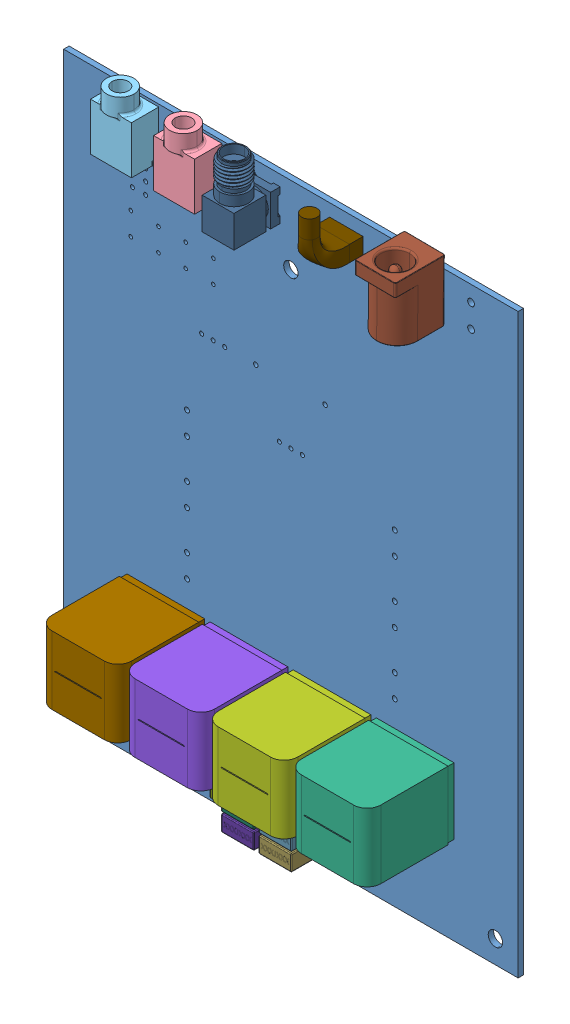
SolidWorks assembly CYAN_AMP_2, configuration 默认. Lengths in mm.
Overall size (100 132.86 23.29).
45 component instances, 18 part files, 2 mates.
Components (placement in the parent):
- CYAN_AMP_2(2)^CYAN_AMP_2-1: CYAN_AMP_2(2)^CYAN_AMP_2 [默认] at origin size (100 132.86 23.29) (virtual)
  - Board^CYAN_AMP_2(2)_CYAN_AMP_2-1: Board^CYAN_AMP_2(2)_CYAN_AMP_2 [默认] at (0 0 -0.8675) size (100 127 1.2) (virtual)
    - board-1: board [默认] at (0 0 -0.4115) size (100 127 1.2)
  - C34^CYAN_AMP_2(2)_CYAN_AMP_2-1: C34^CYAN_AMP_2(2)_CYAN_AMP_2 [默认] at origin (virtual)
    - C_0805^C34_CYAN_AMP_2(2)_CYAN_AMP_2-1: C_0805^C34_CYAN_AMP_2(2)_CYAN_AMP_2 [默认] at (8.9662 61.8782 -0.4115) x (0 1 0) z (0 0 -1) (virtual)
  - LED1^CYAN_AMP_2(2)_CYAN_AMP_2-1: LED1^CYAN_AMP_2(2)_CYAN_AMP_2 [默认] at origin size (3.2 1.6 1.01) (virtual)
    - LED_1206-R^LED1_CYAN_AMP_2(2)_CYAN_AMP_2-1: LED_1206-R^LED1_CYAN_AMP_2(2)_CYAN_AMP_2 [默认] at (11.9888 122.0978 0) x (1 0 0) z (0 0 1) size (3.2 1.6 0.91) (virtual)
      - LED_1206-R-2^LED_1206-R_LED1_CYAN_AMP_2(2)_CYAN_AMP_2-1: LED_1206-R-2^LED_1206-R_LED1_CYAN_AMP_2(2)_CYAN_AMP_2 [默认] at origin size (3.2 1.6 0.91) (virtual)
    - LED_1206glass_RGB255^LED1_CYAN_AMP_2(2)_CYAN_AMP_2-1: LED_1206glass_RGB255^LED1_CYAN_AMP_2(2)_CYAN_AMP_2 [默认] at (11.9888 122.0978 0) x (-1 0 0) z (0 0 1) size (2.25 1.6 0.5) (virtual)
  - JP9^CYAN_AMP_2(2)_CYAN_AMP_2-1: JP9^CYAN_AMP_2(2)_CYAN_AMP_2 [默认] at origin (virtual)
    - KF301^JP9_CYAN_AMP_2(2)_CYAN_AMP_2-2: KF301^JP9_CYAN_AMP_2(2)_CYAN_AMP_2 [默认] at (39.6494 118.5456 0.05) x (0 1 0) z (0 0 1) (virtual)
      - KF301.STEP^KF301_JP9_CYAN_AMP_2(2)_CYAN_AMP_2-1: KF301.STEP^KF301_JP9_CYAN_AMP_2(2)_CYAN_AMP_2 [默认] at origin (virtual)
  - C23^CYAN_AMP_2(2)_CYAN_AMP_2-1: C23^CYAN_AMP_2(2)_CYAN_AMP_2 [默认] at origin (virtual)
    - C_0805^C23_CYAN_AMP_2(2)_CYAN_AMP_2-1: C_0805^C23_CYAN_AMP_2(2)_CYAN_AMP_2 [默认] at (8.9662 66.2216 -0.4115) x (0 -1 0) z (0 0 -1) (virtual)
  - CON3^CYAN_AMP_2(2)_CYAN_AMP_2-1: CON3^CYAN_AMP_2(2)_CYAN_AMP_2 [默认] at origin size (9.19 14 9.05) (virtual)
    - PJ343^CON3_CYAN_AMP_2(2)_CYAN_AMP_2-1: PJ343^CON3_CYAN_AMP_2(2)_CYAN_AMP_2 [默认] at (-19.6067 121.2751 6.0128) x (1 0 0) z (0 1 0) size (9.19 9.05 14) (virtual)
  - CON2^CYAN_AMP_2(2)_CYAN_AMP_2-1: CON2^CYAN_AMP_2(2)_CYAN_AMP_2 [默认] at origin size (9.19 14 9.05) (virtual)
    - PJ343^CON2_CYAN_AMP_2(2)_CYAN_AMP_2-1: PJ343^CON2_CYAN_AMP_2(2)_CYAN_AMP_2 [默认] at (-33.4952 121.2751 6.0128) x (1 0 0) z (0 1 0) size (9.19 9.05 14) (virtual)
  - L4^CYAN_AMP_2(2)_CYAN_AMP_2-1: L4^CYAN_AMP_2(2)_CYAN_AMP_2 [默认] at origin size (17.5 15 22.3) (virtual)
    - 7G17A-C^L4_CYAN_AMP_2(2)_CYAN_AMP_2-1: 7G17A-C^L4_CYAN_AMP_2(2)_CYAN_AMP_2 [默认] at (36.1819 19.2499 1.5) x (-1 0 0) z (0 0 -1) size (17.5 15 22.3) (virtual)
  - L3^CYAN_AMP_2(2)_CYAN_AMP_2-1: L3^CYAN_AMP_2(2)_CYAN_AMP_2 [默认] at origin size (17.5 15 22.3) (virtual)
    - 7G17A-C^L3_CYAN_AMP_2(2)_CYAN_AMP_2-1: 7G17A-C^L3_CYAN_AMP_2(2)_CYAN_AMP_2 [默认] at (17.8939 19.2499 1.5) x (-1 0 0) z (0 0 -1) size (17.5 15 22.3) (virtual)
  - L2^CYAN_AMP_2(2)_CYAN_AMP_2-1: L2^CYAN_AMP_2(2)_CYAN_AMP_2 [默认] at origin size (17.5 15 22.3) (virtual)
    - 7G17A-C^L2_CYAN_AMP_2(2)_CYAN_AMP_2-1: 7G17A-C^L2_CYAN_AMP_2(2)_CYAN_AMP_2 [默认] at (-0.3941 19.2499 1.5) x (-1 0 0) z (0 0 -1) size (17.5 15 22.3) (virtual)
  - L1^CYAN_AMP_2(2)_CYAN_AMP_2-1: L1^CYAN_AMP_2(2)_CYAN_AMP_2 [默认] at origin size (17.5 15 22.3) (virtual)
    - 7G17A-C^L1_CYAN_AMP_2(2)_CYAN_AMP_2-1: 7G17A-C^L1_CYAN_AMP_2(2)_CYAN_AMP_2 [默认] at (-18.6821 19.2499 1.5) x (-1 0 0) z (0 0 -1) size (17.5 15 22.3) (virtual)
  - JP6^CYAN_AMP_2(2)_CYAN_AMP_2-1: JP6^CYAN_AMP_2(2)_CYAN_AMP_2 [默认] at origin size (7 15.1 14.1) (virtual)
    - Samtec-SMA-J-P-H-RA-TH1^JP6_CYAN_AMP_2(2)_CYAN_AMP_2-1: Samtec-SMA-J-P-H-RA-TH1^JP6_CYAN_AMP_2(2)_CYAN_AMP_2 [默认] at (-5.6895 121.2597 0.4) x (-1 0 0) z (0 0 -1) size (7 15.1 14.1) (virtual)
  - CON1^CYAN_AMP_2(2)_CYAN_AMP_2-1: CON1^CYAN_AMP_2(2)_CYAN_AMP_2 [默认] at (26.9848 122.8841 -11.4891) x (-0.999962 0.008727 0) z (0 0 1) size (9.3 14.05 15) (virtual)
    - dc-005.STEP-1: dc-005.STEP [默认] at (-2.5314 0.4154 11.5) size (9.3 14.05 15)
      - dc-005(2)^dc-005.STEP-1: dc-005(2)^dc-005.STEP [默认] at origin size (9.3 14.05 15)
        - DC-005^dc-005(2)_dc-005.STEP-1: DC-005^dc-005(2)_dc-005.STEP [默认] at origin size (9.3 14.05 15)
  - C29^CYAN_AMP_2(2)_CYAN_AMP_2-1: C29^CYAN_AMP_2(2)_CYAN_AMP_2 [默认] at origin size (7.2 3.5 10.9) (virtual)
    - CBB-T_5X7.5X3.5^C29_CYAN_AMP_2(2)_CYAN_AMP_2-1: CBB-T_5X7.5X3.5^C29_CYAN_AMP_2(2)_CYAN_AMP_2 [默认] at (4.0909 2.7138 3.85) x (-1 0 0) z (0 0 -1) size (7.2 3.5 10.9) (virtual)
  - C26^CYAN_AMP_2(2)_CYAN_AMP_2-1: C26^CYAN_AMP_2(2)_CYAN_AMP_2 [默认] at origin size (7.2 5.4 13.4) (virtual)
    - CBB-T_5X10X5.4^C26_CYAN_AMP_2(2)_CYAN_AMP_2-1: CBB-T_5X10X5.4^C26_CYAN_AMP_2(2)_CYAN_AMP_2 [默认] at (4.091 15.8679 5.1127) x (1 0 0) z (0 0 -1) size (7.2 5.4 13.4) (virtual)
  - C24^CYAN_AMP_2(2)_CYAN_AMP_2-1: C24^CYAN_AMP_2(2)_CYAN_AMP_2 [默认] at origin size (7.2 3.5 10.9) (virtual)
    - CBB-T_5X7.5X3.5^C24_CYAN_AMP_2(2)_CYAN_AMP_2-1: CBB-T_5X7.5X3.5^C24_CYAN_AMP_2(2)_CYAN_AMP_2 [默认] at (4.0911 10.1181 3.85) x (1 0 0) z (0 0 -1) size (7.2 3.5 10.9) (virtual)
  - C15^CYAN_AMP_2(2)_CYAN_AMP_2-1: C15^CYAN_AMP_2(2)_CYAN_AMP_2 [默认] at origin size (7.2 3.5 10.9) (virtual)
    - CBB-T_5X7.5X3.5^C15_CYAN_AMP_2(2)_CYAN_AMP_2-1: CBB-T_5X7.5X3.5^C15_CYAN_AMP_2(2)_CYAN_AMP_2 [默认] at (-4.1709 10.1181 3.85) x (1 0 0) z (0 0 -1) size (7.2 3.5 10.9) (virtual)
  - C9^CYAN_AMP_2(2)_CYAN_AMP_2-1: C9^CYAN_AMP_2(2)_CYAN_AMP_2 [默认] at origin size (7.2 5.4 13.4) (virtual)
    - CBB-T_5X10X5.4^C9_CYAN_AMP_2(2)_CYAN_AMP_2-1: CBB-T_5X10X5.4^C9_CYAN_AMP_2(2)_CYAN_AMP_2 [默认] at (-4.171 15.8679 5.1127) x (1 0 0) z (0 0 -1) size (7.2 5.4 13.4) (virtual)
  - C5^CYAN_AMP_2(2)_CYAN_AMP_2-1: C5^CYAN_AMP_2(2)_CYAN_AMP_2 [默认] at origin size (7.2 3.5 10.9) (virtual)
    - CBB-T_5X7.5X3.5^C5_CYAN_AMP_2(2)_CYAN_AMP_2-1: CBB-T_5X7.5X3.5^C5_CYAN_AMP_2(2)_CYAN_AMP_2 [默认] at (-4.1711 2.7138 3.85) x (-1 0 0) z (0 0 -1) size (7.2 3.5 10.9) (virtual)
- 导光柱-1: 导光柱 [默认] at (12.2116 122.5018 -0.079) x (1 0 0) z (0 -1 0) size (7.39 10.05 10.65)
Mates (geometry in assembly coordinates):
- 重合1: coincident: plane of CYAN_AMP_2(2)^CYAN_AMP_2-1/Board^CYAN_AMP_2(2)_CYAN_AMP_2-1/board-1 through (0 0 -0.079) normal (0 0 1); plane of 导光柱-1 through (12.2116 122.5018 -0.079) normal (0 0 -1)
- 重合2: coincident: plane of CYAN_AMP_2(2)^CYAN_AMP_2-1/Board^CYAN_AMP_2(2)_CYAN_AMP_2-1/board-1 through (-50 127 -0.079) normal (0 1 0); circle of 导光柱-1
